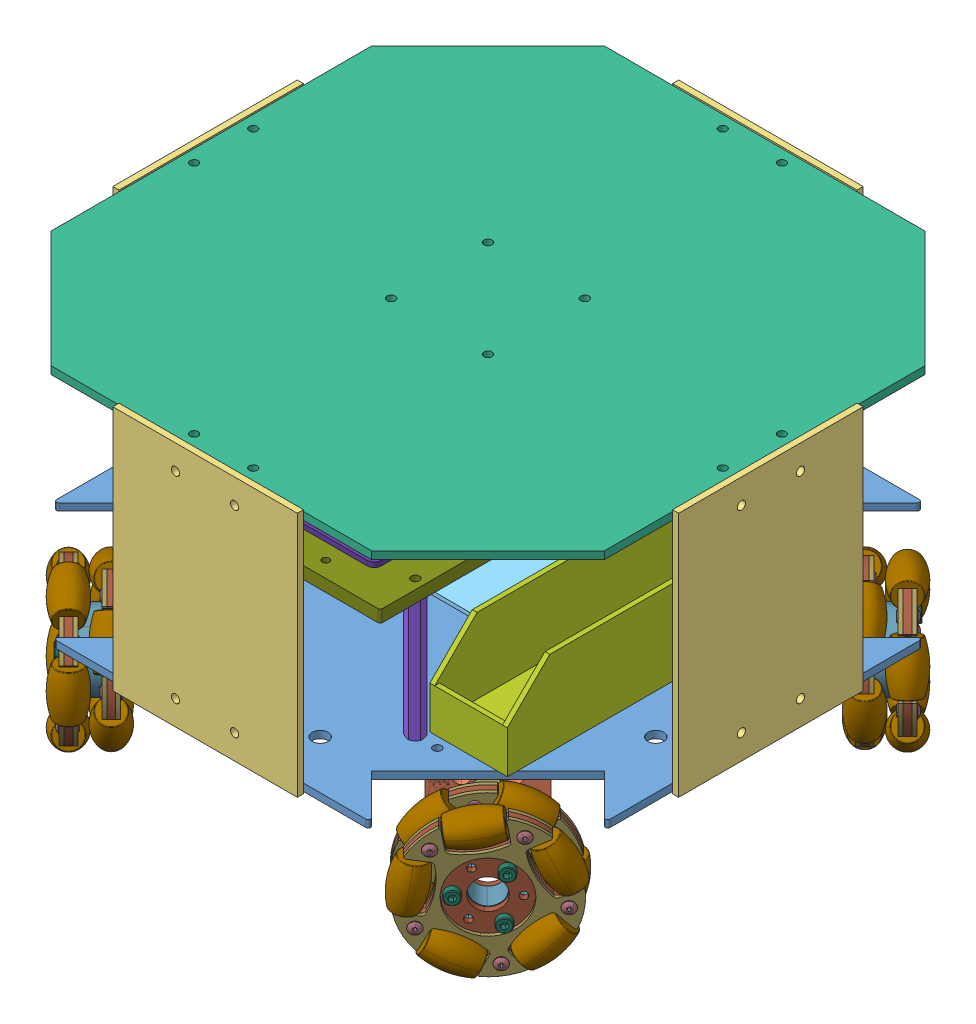
SolidWorks assembly ouijabot, configuration Default. Lengths in mm. (continued)
Components (placement in the parent): (continued)
- wall-1: wall [Default] at (116.84 49.99 0) x (0 0 1) z (0 -1 0) size (76.2 2.54 101.6)
- wall-2: wall [Default] at (0 49.99 116.84) x (-1 0 0) z (0 -1 0) size (76.2 2.54 101.6)
- wall-4: wall [Default] at (-116.84 49.99 0) x (0 0 -1) z (0 -1 0) size (76.2 2.54 101.6)
- wall-7: wall [Default] at (0 49.99 -116.84) x (1 0 0) z (0 -1 0) size (76.2 2.54 101.6)
- motor-controller-holder-arduino-horizontal-1: motor-controller-holder-arduino-horizontal [Default] at (0 3 -60) size (49.8 25 52.8)
- motor-driver-pololu-tb9051ftg-6: motor-driver-pololu-tb9051ftg [Default] at (-24.91 13 -33.59) x (1 0 0) z (0 1 0) size (48.26 51.31 7.67)
- angle-bracket-18: angle-bracket [Default] at (-9.025 96.98 -114.3) x (1 0 0) z (0 -1 0) size (6.35 8.71 9.53)
- angle-bracket-19: angle-bracket [Default] at (15.375 96.98 -114.3) x (1 0 0) z (0 -1 0) size (6.35 8.71 9.53)
- angle-bracket-21: angle-bracket [Default] at (114.3 96.98 -9.025) x (0 0 1) z (0 -1 0) size (6.35 8.71 9.53)
- angle-bracket-23: angle-bracket [Default] at (114.3 96.98 15.375) x (0 0 1) z (0 -1 0) size (6.35 8.71 9.53)
- angle-bracket-25: angle-bracket [Default] at (9.025 96.98 114.3) x (-1 0 0) z (0 -1 0) size (6.35 8.71 9.53)
- angle-bracket-27: angle-bracket [Default] at (-15.375 96.98 114.3) x (-1 0 0) z (0 -1 0) size (6.35 8.71 9.53)
- angle-bracket-29: angle-bracket [Default] at (-114.3 96.98 9.025) x (0 0 -1) z (0 -1 0) size (6.35 8.71 9.53)
- angle-bracket-31: angle-bracket [Default] at (-114.3 96.98 -15.375) x (0 0 -1) z (0 -1 0) size (6.35 8.71 9.53)
- lid-1: lid [Default] at (25.36 96.98 -143.2481) x (-1 0 0) z (0 1 0) size (228.6 228.6 3.17)
Mates (geometry in assembly coordinates):
- Coincident1: coincident: plane of base-1 through (0 0 0) normal (0 -1 0); plane of motor-mount-pololu-1995-1 through (-52.9269 0 78.9485) normal (0 1 0)
- Concentric1: concentric: circle of base-1; circle of motor-mount-pololu-1995-1
- Concentric2: concentric: circle of base-1; circle of motor-mount-pololu-1995-1
- Coincident2: coincident: plane of base-1 through (0 0 0) normal (0 -1 0); plane of motor-mount-pololu-1995-2 through (-78.9485 0 -52.9269) normal (0 1 0)
- Concentric4: concentric: circle of base-1; circle of motor-mount-pololu-1995-2
- Concentric5: concentric: circle of base-1; circle of motor-mount-pololu-1995-2
- Coincident3: coincident: plane of base-1 through (0 0 0) normal (0 -1 0); plane of motor-mount-pololu-1995-3 through (78.9485 0 52.9269) normal (0 1 0)
- Concentric6: concentric: circle of base-1; circle of motor-mount-pololu-1995-3
- Concentric7: concentric: circle of base-1; circle of motor-mount-pololu-1995-3
- Coincident16: coincident: plane of motor-mount-pololu-1995-1 through (-61.3415 -18.4 61.3415) normal (0.707107 0 -0.707107); plane of motor-pololu-2823-1 through (-61.3415 -18.4 61.3415) normal (-0.707107 0 0.707107)
- Concentric16: concentric: cylinder of motor-mount-pololu-1995-1 through (-55.8614 -31.8234 66.8216) axis (0.707107 0 -0.707107) radius 1.65; cylinder of motor-pololu-2823-1 through (-53.8462 -31.8234 64.8063) axis (-0.707107 0 0.707107) radius 1.25
- Concentric17: concentric: cylinder of motor-mount-pololu-1995-1 through (-66.8216 -31.8234 55.8614) axis (0.707107 0 -0.707107) radius 1.65; cylinder of motor-pololu-2823-1 through (-64.8063 -31.8234 53.8462) axis (-0.707107 0 0.707107) radius 1.25
- Coincident17: coincident: plane of motor-mount-pololu-1995-3 through (61.3415 -18.4 61.3415) normal (-0.707107 0 -0.707107); plane of motor-pololu-2823-2 through (61.3415 -18.4 61.3415) normal (0.707107 0 0.707107)
- Concentric18: concentric: cylinder of motor-mount-pololu-1995-3 through (55.8614 -31.8234 66.8216) axis (-0.707107 0 -0.707107) radius 1.65; circle of motor-pololu-2823-2
- Concentric19: concentric: cylinder of motor-mount-pololu-1995-3 through (66.8216 -31.8234 55.8614) axis (-0.707107 0 -0.707107) radius 1.65; cylinder of motor-pololu-2823-2 through (64.8063 -31.8234 53.8462) axis (0.707107 0 0.707107) radius 1.25
- Coincident18: coincident: plane of motor-mount-pololu-1995-2 through (-61.3415 -18.4 -61.3415) normal (0.707107 0 0.707107); plane of motor-pololu-2823-3 through (-61.3415 -18.4 -61.3415) normal (-0.707107 0 -0.707107)
- Concentric20: concentric: circle of motor-mount-pololu-1995-2; circle of motor-pololu-2823-3
- Concentric23: concentric: cylinder of motor-mount-pololu-1995-2 through (-66.8216 -31.8234 -55.8614) axis (0.707107 0 0.707107) radius 1.65; circle of motor-pololu-2823-3
- Coincident19: coincident: plane of base-1 through (0 0 0) normal (0 -1 0); plane of motor-mount-pololu-1995-5 through (52.9269 0 -78.9485) normal (0 1 0)
- Concentric24: concentric: cylinder of base-1 through (74.1048 0 -53.1744) axis (0 1 0) radius 1.7; cylinder of motor-mount-pololu-1995-5 through (74.1048 0 -53.1744) axis (0 1 0) radius 1.25
- Concentric25: concentric: cylinder of base-1 through (53.1744 0 -74.1048) axis (0 1 0) radius 1.7; cylinder of motor-mount-pololu-1995-5 through (53.1744 0 -74.1048) axis (0 1 0) radius 1.25
- Coincident20: coincident: plane of motor-pololu-2823-4 through (61.3415 -18.4 -61.3415) normal (0.707107 0 -0.707107); plane of motor-mount-pololu-1995-5 through (61.3415 -18.4 -61.3415) normal (-0.707107 0 0.707107)
- Concentric26: concentric: cylinder of motor-pololu-2823-4 through (53.8462 -31.8234 -64.8063) axis (0.707107 0 -0.707107) radius 1.25; cylinder of motor-mount-pololu-1995-5 through (55.8614 -31.8234 -66.8216) axis (-0.707107 0 0.707107) radius 1.65
- Concentric28: concentric: cylinder of motor-pololu-2823-4 through (64.8063 -31.8234 -53.8462) axis (0.707107 0 -0.707107) radius 1.25; cylinder of motor-mount-pololu-1995-5 through (66.8216 -31.8234 -55.8614) axis (-0.707107 0 0.707107) radius 1.65
- Coincident24: coincident: plane of base-1 through (0 3 0) normal (0 1 0); plane of standoff-10mm-1 through (-38 3 2.5981) normal (0 -1 0)
- Concentric31: concentric: circle of base-1; circle of standoff-10mm-1
- Concentric32: concentric: circle of base-1; circle of standoff-10mm-2
- Coincident25: coincident: plane of base-1 through (0 3 0) normal (0 1 0); plane of standoff-10mm-2 through (39.3967 3 2.1907) normal (0 -1 0)
- Concentric33: concentric: circle of standoff-10mm-1; circle of protoboard-1
- Concentric36: concentric: circle of standoff-10mm-2; circle of protoboard-1
- Coincident26: coincident: plane of standoff-10mm-1 through (-38 13 2.5981) normal (0 1 0); plane of protoboard-1 through (0 13 0) normal (0 -1 0)
- Concentric37: concentric: cylinder of angle-bracket-1 through (109.1438 2.999 12.2) axis (0 1 0) radius 1.651; cylinder of base-1 through (109.1438 -0.001 12.2) axis (0 1 0) radius 1.7
- Coincident27: coincident: plane of base-1 through (0 3 0) normal (0 1 0); plane of angle-bracket-1 through (114.3 3 15.375) normal (0 -1 0)
- Coincident28: coincident: plane of base-1 through (0 3 0) normal (0 1 0); plane of angle-bracket-2 through (114.3 3 -9.025) normal (0 -1 0)
- Concentric38: concentric: cylinder of angle-bracket-2 through (109.1438 2.999 -12.2) axis (0 1 0) radius 1.651; cylinder of base-1 through (109.1438 -0.001 -12.2) axis (0 1 0) radius 1.7
- Parallel5: parallel: plane of base-1 through (114.3 3 -114.3) normal (1 0 0); plane of angle-bracket-2 through (114.3 12.525 -9.025) normal (1 0 0)
- Parallel6: parallel: plane of base-1 through (114.3 3 -114.3) normal (1 0 0); plane of angle-bracket-1 through (114.3 12.525 15.375) normal (1 0 0)
- Concentric39: concentric: cylinder of base-1 through (12.2 -0.001 -109.1438) axis (0 1 0) radius 1.7; cylinder of angle-bracket-4 through (12.2 2.999 -109.1438) axis (0 1 0) radius 1.651
- Coincident32: coincident: plane of base-1 through (0 3 0) normal (0 1 0); plane of angle-bracket-4 through (15.375 3 -114.3) normal (0 -1 0)
- Parallel7: parallel: plane of base-1 through (-114.3 3 -114.3) normal (0 0 -1); plane of angle-bracket-4 through (15.375 12.525 -114.3) normal (0 0 -1)
- Concentric40: concentric: cylinder of base-1 through (-12.2 -0.001 -109.1438) axis (0 1 0) radius 1.7; cylinder of angle-bracket-6 through (-12.2 2.999 -109.1438) axis (0 1 0) radius 1.651
- Coincident33: coincident: plane of base-1 through (0 3 0) normal (0 1 0); plane of angle-bracket-6 through (-9.025 3 -114.3) normal (0 -1 0)
- Parallel8: parallel: plane of base-1 through (-114.3 3 -114.3) normal (0 0 -1); plane of angle-bracket-6 through (-9.025 12.525 -114.3) normal (0 0 -1)
- Concentric41: concentric: cylinder of angle-bracket-8 through (-109.1438 2.999 -12.2) axis (0 1 0) radius 1.651; cylinder of base-1 through (-109.1438 -0.001 -12.2) axis (0 1 0) radius 1.7
- Coincident34: coincident: plane of base-1 through (0 3 0) normal (0 1 0); plane of angle-bracket-8 through (-114.3 3 -15.375) normal (0 -1 0)
- Parallel9: parallel: plane of base-1 through (-114.3 3 -114.3) normal (-1 0 0); plane of angle-bracket-8 through (-114.3 12.525 -15.375) normal (-1 0 0)
- Concentric42: concentric: cylinder of angle-bracket-10 through (-109.1438 2.999 12.2) axis (0 1 0) radius 1.651; cylinder of base-1 through (-109.1438 -0.001 12.2) axis (0 1 0) radius 1.7
- Coincident35: coincident: plane of base-1 through (0 3 0) normal (0 1 0); plane of angle-bracket-10 through (-114.3 3 9.025) normal (0 -1 0)
- Parallel10: parallel: plane of base-1 through (-114.3 3 -114.3) normal (-1 0 0); plane of angle-bracket-10 through (-114.3 12.525 9.025) normal (-1 0 0)
- Coincident36: coincident: plane of base-1 through (0 3 0) normal (0 1 0); plane of angle-bracket-12 through (-15.375 3 114.3) normal (0 -1 0)
- Parallel12: parallel: plane of base-1 through (-114.3 3 114.3) normal (0 0 1); plane of angle-bracket-12 through (-15.375 12.525 114.3) normal (0 0 1)
- Coincident37: coincident: plane of base-1 through (0 3 0) normal (0 1 0); plane of angle-bracket-14 through (9.025 3 114.3) normal (0 -1 0)
- Parallel13: parallel: plane of base-1 through (-114.3 3 114.3) normal (0 0 1); plane of angle-bracket-14 through (9.025 12.525 114.3) normal (0 0 1)
- Distance2: distance = 3.1 mm: plane of base-1 through (0 3 0) normal (0 1 0); plane of battery-holder-1 through (-65 6.1 0) normal (0 -1 0)
- Concentric47: concentric: cylinder of base-1 through (-65 -0.001 -30) axis (0 1 0) radius 1.7; cylinder of battery-holder-1 through (-65 6.099 -30) axis (0 1 0) radius 1.7
- Concentric48: concentric: cylinder of base-1 through (-65 -0.001 30) axis (0 1 0) radius 1.7; cylinder of battery-holder-1 through (-65 6.099 30) axis (0 1 0) radius 1.7
- Distance3: distance = 3.1 mm: plane of base-1 through (0 3 0) normal (0 1 0); plane of battery-holder-2 through (65 6.1 0) normal (0 -1 0)
- Concentric49: concentric: cylinder of base-1 through (65 -0.001 -30) axis (0 1 0) radius 1.7; cylinder of battery-holder-2 through (65 6.099 -30) axis (0 1 0) radius 1.7
- Concentric50: concentric: circle of base-1; cylinder of battery-holder-2 through (65 6.099 30) axis (0 1 0) radius 1.7
- Coincident40: coincident: plane of base-1 through (0 3 0) normal (0 1 0); plane of standoff-51mm-1 through (-44 3 77.4641) normal (0 -1 0)
- Concentric51: concentric: circle of base-1; circle of standoff-51mm-1
- Coincident41: coincident: plane of base-1 through (0 3 0) normal (0 1 0); plane of standoff-51mm-2 through (44.6528 3 77.402) normal (0 -1 0)
- Concentric52: concentric: circle of base-1; circle of standoff-51mm-2
- Coincident42: coincident: plane of base-1 through (0 3 0) normal (0 1 0); plane of standoff-51mm-4 through (45.3709 3 -70.8187) normal (0 -1 0)
- Concentric53: concentric: circle of base-1; circle of standoff-51mm-4
- Coincident43: coincident: plane of base-1 through (0 3 0) normal (0 1 0); plane of standoff-51mm-6 through (-41.9215 3 -71.2287) normal (0 -1 0)
- Concentric54: concentric: circle of base-1; circle of standoff-51mm-6
- Concentric55: concentric: cylinder of motor-pololu-2823-3 through (-76.8979 -25.4 -76.8979) axis (0.707107 0 0.707107) radius 3; cylinder of omni-wheel-60mm-1/(Nex) [RB-Nex-75] [14145] 60mm Aluminum Omni Wheel - SolidWorks Model.STEP-1/60mm90__5______-______________(A__ ).STEP-2/60mm90__5______-____________(A__).STEP-1 through (-76.8979 -25.4 -76.8979) axis (-0.707107 0 -0.707107) radius 6.25
- Distance1: distance = 16 mm: plane of omni-wheel-60mm-1/(Nex) [RB-Nex-75] [14145] 60mm Aluminum Omni Wheel - SolidWorks Model.STEP-1/60mm90__5______-______________(A__ ).STEP-2/60mm90__5______-____________(A__).STEP-1 through (-76.8979 -25.4 -76.8979) normal (0.707107 0 0.707107); plane of motor-pololu-2823-3 through (-65.5842 -18.4 -65.5842) normal (-0.707107 0 -0.707107)
- Concentric57: concentric: cylinder of motor-pololu-2823-4 through (76.8979 -25.4 -76.8979) axis (-0.707107 0 0.707107) radius 3; cylinder of omni-wheel-60mm-2/(Nex) [RB-Nex-75] [14145] 60mm Aluminum Omni Wheel - SolidWorks Model.STEP-1/60mm90__5______-______________(A__ ).STEP-2/60mm90__5______-____________(A__).STEP-1 through (76.8979 -25.4 -76.8979) axis (0.707107 0 -0.707107) radius 6.25
- Distance4: distance = 16 mm: plane of omni-wheel-60mm-2/(Nex) [RB-Nex-75] [14145] 60mm Aluminum Omni Wheel - SolidWorks Model.STEP-1/60mm90__5______-______________(A__ ).STEP-2/60mm90__5______-____________(A__).STEP-1 through (76.8979 -25.4 -76.8979) normal (-0.707107 0 0.707107); plane of motor-pololu-2823-4 through (65.5842 -18.4 -65.5842) normal (0.707107 0 -0.707107)
- Concentric58: concentric: cylinder of motor-pololu-2823-2 through (76.8979 -25.4 76.8979) axis (-0.707107 0 -0.707107) radius 3; cylinder of omni-wheel-60mm-4/(Nex) [RB-Nex-75] [14145] 60mm Aluminum Omni Wheel - SolidWorks Model.STEP-1/60mm90__5______-______________(A__ ).STEP-2/60mm90__5______-____________(A__).STEP-1 through (76.8979 -25.4 76.8979) axis (0.707107 0 0.707107) radius 6.25
- Distance5: distance = 16 mm: plane of omni-wheel-60mm-4/(Nex) [RB-Nex-75] [14145] 60mm Aluminum Omni Wheel - SolidWorks Model.STEP-1/60mm90__5______-______________(A__ ).STEP-2/60mm90__5______-____________(A__).STEP-1 through (76.8979 -25.4 76.8979) normal (-0.707107 0 -0.707107); plane of motor-pololu-2823-2 through (65.5842 -18.4 65.5842) normal (0.707107 0 0.707107)
- Concentric59: concentric: cylinder of motor-pololu-2823-1 through (-76.8979 -25.4 76.8979) axis (0.707107 0 -0.707107) radius 3; cylinder of omni-wheel-60mm-6/(Nex) [RB-Nex-75] [14145] 60mm Aluminum Omni Wheel - SolidWorks Model.STEP-1/60mm90__5______-______________(A__ ).STEP-2/60mm90__5______-____________(A__).STEP-1 through (-76.8979 -25.4 76.8979) axis (-0.707107 0 0.707107) radius 6.25
- Distance6: distance = 16 mm: plane of omni-wheel-60mm-6/(Nex) [RB-Nex-75] [14145] 60mm Aluminum Omni Wheel - SolidWorks Model.STEP-1/60mm90__5______-______________(A__ ).STEP-2/60mm90__5______-____________(A__).STEP-1 through (-76.8979 -25.4 76.8979) normal (0.707107 0 -0.707107); plane of motor-pololu-2823-1 through (-65.5842 -18.4 65.5842) normal (-0.707107 0 0.707107)
- Concentric60: concentric: circle of standoff-51mm-6; cylinder of level2-plate-1 through (-44 53.999 -74) axis (0 1 0) radius 1.7
- Concentric61: concentric: circle of standoff-51mm-2; cylinder of level2-plate-1 through (44 53.999 74) axis (0 1 0) radius 1.7
- Coincident44: coincident: plane of standoff-51mm-4 through (45.3709 54 -70.8187) normal (0 1 0); plane of level2-plate-1 through (0 54 0) normal (0 -1 0)
- Coincident45: coincident: plane of level2-plate-1 through (0 59 0) normal (0 1 0); plane of standoff-10mm-3 through (-38 59 2.5981) normal (0 -1 0)
- Concentric62: concentric: circle of level2-plate-1; circle of standoff-10mm-3
- Coincident46: coincident: plane of level2-plate-1 through (0 59 0) normal (0 1 0); plane of standoff-10mm-4 through (38.4896 59 2.5515) normal (0 -1 0)
- Concentric63: concentric: circle of level2-plate-1; circle of standoff-10mm-4
- Coincident47: coincident: plane of standoff-10mm-3 through (-38 69 2.5981) normal (0 1 0); plane of protoboard-2 through (0 69 0) normal (0 -1 0)
- Concentric64: concentric: circle of standoff-10mm-4; cylinder of protoboard-2 through (38 68.999 0) axis (0 1 0) radius 1.778
- Concentric65: concentric: circle of standoff-10mm-3; circle of protoboard-2
- Distance7: distance = 10 mm: plane of raspberry_pi-1 through (0 69 61.48) normal (0 -1 0); plane of level2-plate-1 through (0 59 0) normal (0 1 0)
- Parallel14: parallel: plane of level2-plate-1 through (-48 59 -92.5) normal (-1 0 0); plane of raspberry_pi-1 through (-42.5 71 33.48) normal (-1 0 0)
- Width1: width: plane of raspberry_pi-1 through (-42.5 71 33.48) normal (-1 0 0); plane of raspberry_pi-1 through (42.5 71 33.48) normal (1 0 0); plane of level2-plate-1 through (-48 59 -92.5) normal (-1 0 0); plane of level2-plate-1 through (48 59 -92.5) normal (1 0 0)
- Distance8: distance = 3 mm: plane of raspberry_pi-1 through (-42.5 71 33.48) normal (0 0 -1); plane of protoboard-2 through (-43.18 70.6 30.48) normal (0 0 1)
- Distance10: distance = 15 mm: plane of level2-plate-1 through (0 59 0) normal (0 1 0); plane of tx2-carrier-orbitty-1/ASG003_3D_MODEL.step-1/Board.step-1 through (43.5 74 -33.48) normal (0 -1 0)
- Width2: width: plane of tx2-carrier-orbitty-1/ASG003_3D_MODEL.step-1/Board.step-1 through (43.5 75.6006 -83.48) normal (1 0 0); plane of tx2-carrier-orbitty-1/ASG003_3D_MODEL.step-1/Board.step-1 through (-43.5 75.6006 -33.48) normal (-1 0 0); plane of level2-plate-1 through (48 59 -92.5) normal (1 0 0); plane of level2-plate-1 through (-48 59 -92.5) normal (-1 0 0)
- Distance11: distance = 3 mm: plane of tx2-carrier-orbitty-1/ASG003_3D_MODEL.step-1/Board.step-1 through (43.5 75.6006 -33.48) normal (0 0 1); plane of protoboard-2 through (-43.18 70.6 -30.48) normal (0 0 -1)
- Coincident50: coincident: plane of angle-bracket-2 through (114.3 12.525 -9.025) normal (1 0 0); plane of wall-1 through (114.3 49.99 0) normal (-1 0 0)
- Concentric66: concentric: cylinder of angle-bracket-2 through (114.301 9.35 -12.2) axis (-1 0 0) radius 1.4224; cylinder of wall-1 through (114.3 9.35 -12.2) axis (1 0 0) radius 1.7
- Concentric67: concentric: circle of angle-bracket-1; cylinder of wall-1 through (114.3 9.35 12.2) axis (1 0 0) radius 1.7
- Coincident51: coincident: plane of angle-bracket-12 through (-15.375 12.525 114.3) normal (0 0 1); plane of wall-2 through (0 49.99 114.3) normal (0 0 -1)
- Concentric68: concentric: circle of angle-bracket-14; cylinder of wall-2 through (12.2 9.35 114.3) axis (0 0 1) radius 1.7
- Concentric69: concentric: circle of angle-bracket-12; cylinder of wall-2 through (-12.2 9.35 114.3) axis (0 0 1) radius 1.7
- Coincident52: coincident: plane of angle-bracket-10 through (-114.3 12.525 9.025) normal (-1 0 0); plane of wall-4 through (-114.3 49.99 0) normal (1 0 0)
- Concentric70: concentric: cylinder of angle-bracket-10 through (-114.301 9.35 12.2) axis (1 0 0) radius 1.4224; cylinder of wall-4 through (-114.3 9.35 12.2) axis (-1 0 0) radius 1.7
- Concentric71: concentric: cylinder of angle-bracket-8 through (-114.301 9.35 -12.2) axis (1 0 0) radius 1.4224; cylinder of wall-4 through (-114.3 9.35 -12.2) axis (-1 0 0) radius 1.7
- Coincident54: coincident: plane of angle-bracket-6 through (-9.025 12.525 -114.3) normal (0 0 -1); plane of wall-7 through (0 49.99 -114.3) normal (0 0 1)
- Concentric72: concentric: cylinder of angle-bracket-6 through (-12.2 9.35 -114.301) axis (0 0 1) radius 1.4224; cylinder of wall-7 through (-12.2 9.35 -114.3) axis (0 0 -1) radius 1.7
- Concentric73: concentric: cylinder of angle-bracket-4 through (12.2 9.35 -114.301) axis (0 0 1) radius 1.4224; cylinder of wall-7 through (12.2 9.35 -114.3) axis (0 0 -1) radius 1.7
- Concentric81: concentric: cylinder of base-1 through (12.2 -0.001 109.1438) axis (0 1 0) radius 1.7; cylinder of angle-bracket-14 through (12.2 2.999 109.1438) axis (0 1 0) radius 1.651
- Concentric82: concentric: cylinder of base-1 through (-12.2 -0.001 109.1438) axis (0 1 0) radius 1.7; cylinder of angle-bracket-12 through (-12.2 2.999 109.1438) axis (0 1 0) radius 1.651
- Concentric83: concentric: cylinder of base-1 through (-109.1438 -0.001 -12.2) axis (0 1 0) radius 1.7; circle of angle-bracket-8
- Concentric84: concentric: cylinder of base-1 through (-109.1438 -0.001 12.2) axis (0 1 0) radius 1.7; cylinder of angle-bracket-10 through (-109.1438 2.999 12.2) axis (0 1 0) radius 1.651
- Coincident55: coincident: plane of base-1 through (0 3 0) normal (0 1 0); plane of motor-controller-holder-arduino-horizontal-1 through (0 3 -60) normal (0 -1 0)
- Concentric85: concentric: circle of base-1; circle of motor-controller-holder-arduino-horizontal-1
- Concentric86: concentric: circle of base-1; circle of motor-controller-holder-arduino-horizontal-1
- Coincident58: coincident: plane of motor-controller-holder-arduino-horizontal-1 through (0 13 -60) normal (0 1 0); plane of motor-driver-pololu-tb9051ftg-6 through (-24.91 13 -33.59) normal (0 -1 0)
- Concentric87: concentric: circle of motor-controller-holder-arduino-horizontal-1; circle of motor-driver-pololu-tb9051ftg-6
- Parallel15: parallel: plane of motor-controller-holder-arduino-horizontal-1 through (0 28 -85.15) normal (0 0 1); plane of motor-driver-pololu-tb9051ftg-6 through (23.35 14.5748 -84.898) normal (0 0 -1)
- Coincident62: coincident: plane of wall-7 through (0 49.99 -114.3) normal (0 0 1); plane of angle-bracket-18 through (-15.375 87.455 -114.3) normal (0 0 -1)
- Concentric90: concentric: cylinder of wall-7 through (-12.2 90.63 -114.3) axis (0 0 -1) radius 1.7; cylinder of angle-bracket-18 through (-12.2 90.63 -114.301) axis (0 0 1) radius 1.4224
- Parallel17: parallel: plane of wall-7 through (-38.1 100.79 -114.3) normal (0 1 0); plane of angle-bracket-18 through (-15.375 96.98 -114.3) normal (0 1 0)
- Coincident64: coincident: plane of wall-7 through (0 49.99 -114.3) normal (0 0 1); plane of angle-bracket-19 through (9.025 87.455 -114.3) normal (0 0 -1)
- Concentric91: concentric: circle of wall-7; cylinder of angle-bracket-19 through (12.2 90.63 -114.301) axis (0 0 1) radius 1.4224
- Parallel18: parallel: plane of wall-7 through (-38.1 100.79 -114.3) normal (0 1 0); plane of angle-bracket-19 through (9.025 96.98 -114.3) normal (0 1 0)
- Coincident65: coincident: plane of wall-1 through (114.3 49.99 0) normal (-1 0 0); plane of angle-bracket-21 through (114.3 87.455 -15.375) normal (1 0 0)
- Concentric92: concentric: circle of wall-1; cylinder of angle-bracket-21 through (114.301 90.63 -12.2) axis (-1 0 0) radius 1.4224
- Parallel19: parallel: plane of wall-1 through (114.3 100.79 -38.1) normal (0 1 0); plane of angle-bracket-21 through (114.3 96.98 -15.375) normal (0 1 0)
- Coincident66: coincident: plane of wall-1 through (114.3 49.99 0) normal (-1 0 0); plane of angle-bracket-23 through (114.3 87.455 9.025) normal (1 0 0)
- Concentric93: concentric: cylinder of wall-1 through (114.3 90.63 12.2) axis (1 0 0) radius 1.7; cylinder of angle-bracket-23 through (114.301 90.63 12.2) axis (-1 0 0) radius 1.4224
- Parallel20: parallel: plane of wall-1 through (114.3 100.79 -38.1) normal (0 1 0); plane of angle-bracket-23 through (114.3 96.98 9.025) normal (0 1 0)
- Concentric94: concentric: circle of wall-2; cylinder of angle-bracket-25 through (12.2 90.63 114.301) axis (0 0 -1) radius 1.4224
- Parallel21: parallel: plane of wall-2 through (38.1 100.79 114.3) normal (0 1 0); plane of angle-bracket-25 through (15.375 96.98 114.3) normal (0 1 0)
- Coincident68: coincident: plane of wall-2 through (0 49.99 114.3) normal (0 0 -1); plane of angle-bracket-27 through (-9.025 87.455 114.3) normal (0 0 1)
- Concentric95: concentric: cylinder of wall-2 through (-12.2 90.63 114.3) axis (0 0 1) radius 1.7; cylinder of angle-bracket-27 through (-12.2 90.63 114.301) axis (0 0 -1) radius 1.4224
- Parallel22: parallel: plane of wall-2 through (38.1 100.79 114.3) normal (0 1 0); plane of angle-bracket-27 through (-9.025 96.98 114.3) normal (0 1 0)
- Coincident69: coincident: plane of wall-4 through (-114.3 49.99 0) normal (1 0 0); plane of angle-bracket-29 through (-114.3 87.455 15.375) normal (-1 0 0)
- Concentric96: concentric: cylinder of wall-4 through (-114.3 90.63 12.2) axis (-1 0 0) radius 1.7; cylinder of angle-bracket-29 through (-114.301 90.63 12.2) axis (1 0 0) radius 1.4224
- Parallel23: parallel: plane of wall-4 through (-114.3 100.79 38.1) normal (0 1 0); plane of angle-bracket-29 through (-114.3 96.98 15.375) normal (0 1 0)
- Coincident70: coincident: plane of wall-4 through (-114.3 49.99 0) normal (1 0 0); plane of angle-bracket-31 through (-114.3 87.455 -9.025) normal (-1 0 0)
- Concentric97: concentric: cylinder of wall-4 through (-114.3 90.63 -12.2) axis (-1 0 0) radius 1.7; cylinder of angle-bracket-31 through (-114.301 90.63 -12.2) axis (1 0 0) radius 1.4224
- Parallel24: parallel: plane of wall-4 through (-114.3 100.79 38.1) normal (0 1 0); plane of angle-bracket-31 through (-114.3 96.98 -9.025) normal (0 1 0)
- Coincident71: coincident: plane of wall-2 through (0 49.99 114.3) normal (0 0 -1); plane of angle-bracket-25 through (15.375 87.455 114.3) normal (0 0 1)
- Coincident72: coincident: plane of angle-bracket-23 through (114.3 96.98 9.025) normal (0 1 0); plane of lid-1 through (25.36 96.98 -143.2481) normal (0 -1 0)
- Parallel25: parallel: plane of wall-4 through (-114.3 49.99 0) normal (1 0 0); plane of lid-1 through (-114.3 100.155 -143.2481) normal (-1 0 0)
- Width3: width: plane of wall-4 through (-114.3 49.99 0) normal (1 0 0); plane of wall-1 through (114.3 49.99 0) normal (-1 0 0); plane of lid-1 through (-114.3 100.155 -143.2481) normal (-1 0 0); plane of lid-1 through (114.3 100.155 -143.2481) normal (1 0 0)
- Width4: width: plane of wall-7 through (0 49.99 -114.3) normal (0 0 1); plane of wall-2 through (0 49.99 114.3) normal (0 0 -1); plane of lid-1 through (25.36 100.155 -114.3) normal (0 0 -1); plane of lid-1 through (25.36 100.155 114.3) normal (0 0 1)
